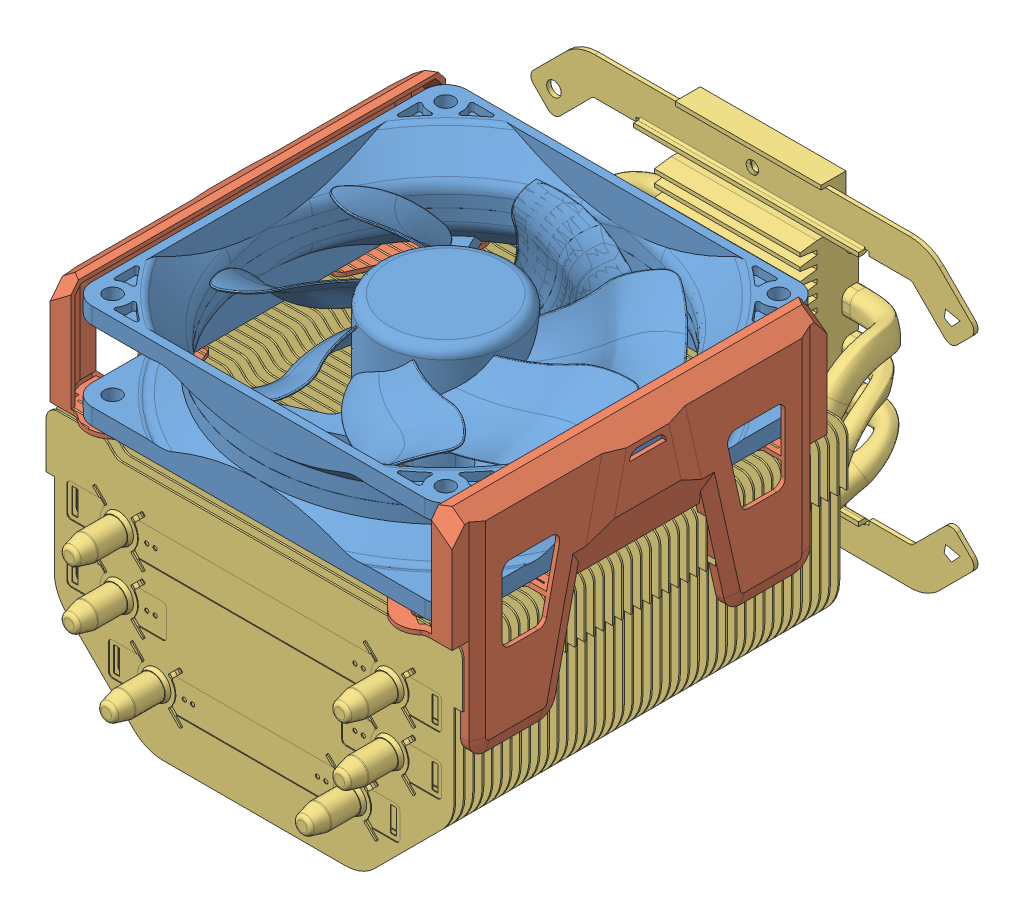
SolidWorks assembly 7030028_ASSY_CPU HEATSINK.igs, configuration Default. Lengths in mm.
Overall size (108.44 87.6 180.01).
4 component instances, 3 part files, 0 mates.
Components (placement in the parent):
- 7030025_PART_FAN STANDARD 90_MODEL.igs-1: 7030025_PART_FAN STANDARD 90_MODEL.igs [Default] at (0 45 -45) x (1 0 0) z (0 -1 0) size (93.98 180.01 25.07)
- 7030026_PART_HEATSINK ADAPTOR 90_MODEL.igs-1: 7030026_PART_HEATSINK ADAPTOR 90_MODEL.igs [Default] at (95 58.5 47.4641) x (0 0 -1) z (-1 0 0) size (106.39 52.6 26.58)
- 7030026_PART_HEATSINK ADAPTOR 90_MODEL.igs-2: 7030026_PART_HEATSINK ADAPTOR 90_MODEL.igs [Default] at (-7 58.5 -46) x (0 0 1) z (1 0 0) size (106.39 52.6 26.58)
- 7030027_PART_CPU HEATSINK TOWER_MODEL.igs-1: 7030027_PART_CPU HEATSINK TOWER_MODEL.igs [Default] at (94 31.5 -47.65) x (-1 0 0) z (0 0 1) size (108.44 80.01 139.76)
